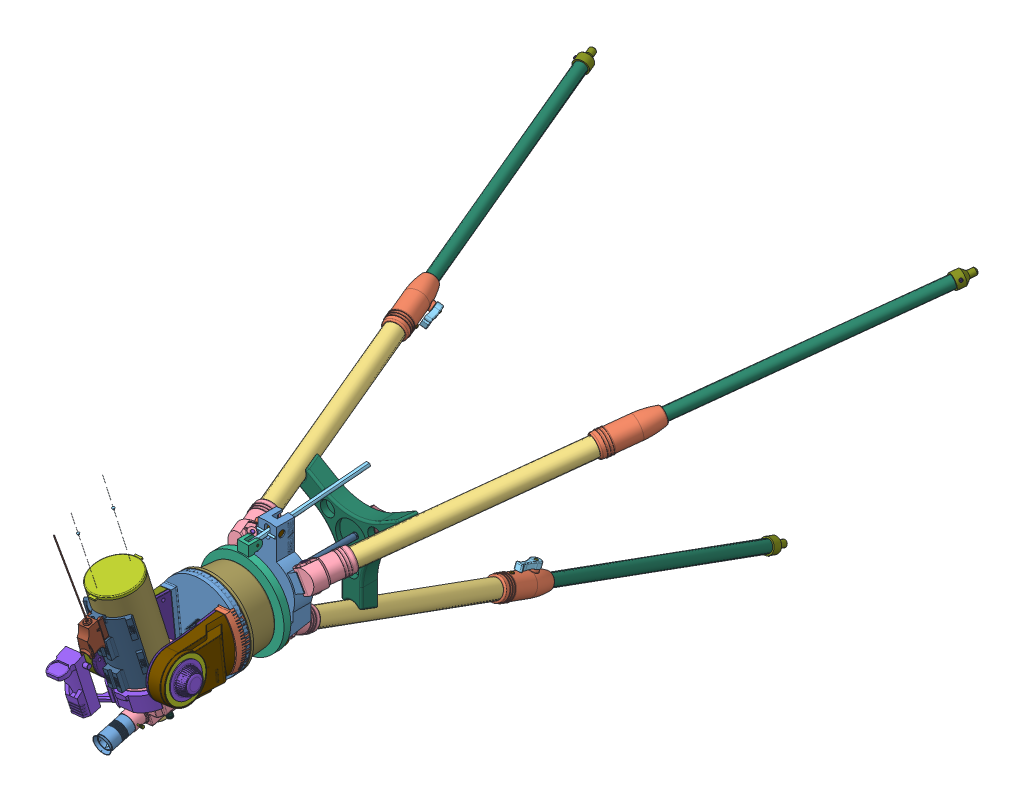
SolidWorks assembly trepied, configuration Défaut. Lengths in mm.
Overall size (885.88 767.19 1585.6).
256 component instances, 124 part files, 38 mates.
Components (placement in the parent):
- plateforme trepied-1: plateforme trepied [Défaut] at (-13.9917 -19.2932 0) size (184.28 220 78.5)
- tube superieur-1: tube superieur [Défaut] at (-47.7776 -290.931 -548.273) x (-1 0 0) z (0 -0.939693 0.34202) size (56 647 70.31)
  - liaison tube-1: liaison tube [Défaut] at (-33.7859 -53.3876 0) size (49 123 52)
  - tube superieur-1: tube superieur [Défaut] at (-33.7859 -3.3876 0) x (1 0 0) z (0 -1 0) size (38 38 530)
  - liaison tube plaque-1: liaison tube plaque [Défaut] at (-33.7859 -483.3876 0) x (-1 0 0) z (0 0 1) size (54 94 52.5)
  - manette fixation pied-1: manette fixation pied [Défaut] at (-52.9516 19.4533 -40.9) x (-1 0 0) z (0 0 1) size (22 50 29.31)
    - manette fixation pied-1: manette fixation pied [Défaut] at (-19.1657 -10.1591 0) size (22 50 15.3)
    - vis M8 fixation pied-1: vis M8 fixation pied [Défaut] at (-19.1657 -10.1591 6.2) x (1 0 0) z (0 -1 0) size (11 21.7 11)
    - Vis cr f90 M4-1: Vis cr f90 M4 [Défaut] at (-19.1657 -10.1591 1.7) size (7.4 7.4 13.11)
  - VisChcM8 50-2: VisChcM8 50 [Défaut] at (-55.5859 -557.3876 0) x (0 0 -1) z (1 0 0) size (12.3 12.3 56)
  - Vis cr M5-1: Vis cr M5 [Défaut] at (-33.7859 -20.3876 -23.15) x (0 1 0) z (0 0 1) size (7.7 7.7 9.33)
  - Vis cr M5-2: Vis cr M5 [Défaut] at (-33.7859 -516.3876 -23.15) size (7.7 7.7 9.33)
- axe M12-1: axe M12 [Défaut] at (-13.9917 -19.2932 0) x (-0.923728 -0.383049 0) z (0 0 -1) size (12.15 12.3 255.78)
- rondelle 30-1: rondelle 30 [Défaut] at (-13.9917 -19.2932 -220.4136) x (0.988696 -0.149935 0) z (0 0 1) size (30 30 2.3)
- Ecrou hexagonal ISO 4032, M 12-1: Ecrou hexagonal ISO 4032, M 12 [Défaut] at (-13.9917 -19.2932 -29.8) x (0.5 0.866025 0) z (0.866025 -0.5 0) size (20.78 10.8 18)
- ecrou plastic M12-1: ecrou plastic M12 [Défaut] at (-30.5314 -30.6977 -251.8636) x (-0.809017 -0.587785 0) z (0 0 1) size (58 55.29 30.73)
  - ecrou plastic-1: ecrou plastic [Défaut] at (-20.0843 0.4954 0) size (58 55.29 30)
  - insert M12-1: insert M12 [Défaut] at (-20.0843 0.4954 14.3) size (16 16 17.46)
- pied-1: pied [Défaut] at (-11.1207 -290.7802 -547.9154) x (1 0 0) z (0 -0.34202 -0.939693) size (30.8 33.14 626.85)
  - tube inferieur-1: tube inferieur [Défaut] at (-2.871 0.0194 0) size (25 25 600)
  - pied-1: pied [Défaut] at (-2.871 0.0194 582.85) x (1 0 0) z (0 -1 0) size (30.8 44 30.8)
  - Vis cr M4-1: Vis cr M4 [Défaut] at (-2.871 15.3194 591.85) x (0 0 -1) z (0 -1 0) size (6.7 6.7 12.44)
- pied-2: pied [Défaut] at (-250.5418 113.9639 -547.9154) x (-0.5 -0.866025 0) z (-0.296198 0.17101 -0.939693) size (30.8 33.14 626.85)
  - tube inferieur-1: tube inferieur [Défaut] at (-2.871 0.0194 0) size (25 25 600)
  - pied-1: pied [Défaut] at (-2.871 0.0194 582.85) x (1 0 0) z (0 -1 0) size (30.8 44 30.8)
  - Vis cr M4-1: Vis cr M4 [Défaut] at (-2.871 15.3194 591.85) x (0 0 -1) z (0 -1 0) size (6.7 6.7 12.44)
- pied-3: pied [Défaut] at (219.6874 118.9366 -547.9154) x (-0.5 0.866025 0) z (0.296198 0.17101 -0.939693) size (30.8 33.14 626.85)
  - tube inferieur-1: tube inferieur [Défaut] at (-2.871 0.0194 0) size (25 25 600)
  - pied-1: pied [Défaut] at (-2.871 0.0194 582.85) x (1 0 0) z (0 -1 0) size (30.8 44 30.8)
  - Vis cr M4-1: Vis cr M4 [Défaut] at (-2.871 15.3194 591.85) x (0 0 -1) z (0 -1 0) size (6.7 6.7 12.44)
- tube superieur-2: tube superieur [Défaut] at (-232.344 145.7851 -548.273) x (0.5 0.866025 0) z (-0.813798 0.469846 0.34202) size (56 647 70.31)
  - liaison tube-1: liaison tube [Défaut] at (-33.7859 -53.3876 0) size (49 123 52)
  - tube superieur-1: tube superieur [Défaut] at (-33.7859 -3.3876 0) x (1 0 0) z (0 -1 0) size (38 38 530)
  - liaison tube plaque-1: liaison tube plaque [Défaut] at (-33.7859 -483.3876 0) x (-1 0 0) z (0 0 1) size (54 94 52.5)
  - manette fixation pied-1: manette fixation pied [Défaut] at (-52.9516 19.4533 -40.9) x (-1 0 0) z (0 0 1) size (22 50 29.31)
    - manette fixation pied-1: manette fixation pied [Défaut] at (-19.1657 -10.1591 0) size (22 50 15.3)
    - vis M8 fixation pied-1: vis M8 fixation pied [Défaut] at (-19.1657 -10.1591 6.2) x (1 0 0) z (0 -1 0) size (11 21.7 11)
    - Vis cr f90 M4-1: Vis cr f90 M4 [Défaut] at (-19.1657 -10.1591 1.7) size (7.4 7.4 13.11)
  - VisChcM8 50-2: VisChcM8 50 [Défaut] at (-55.5859 -557.3876 0) x (0 0 -1) z (1 0 0) size (12.3 12.3 56)
  - Vis cr M5-1: Vis cr M5 [Défaut] at (-33.7859 -20.3876 -23.15) x (0 1 0) z (0 0 1) size (7.7 7.7 9.33)
  - Vis cr M5-2: Vis cr M5 [Défaut] at (-33.7859 -516.3876 -23.15) size (7.7 7.7 9.33)
- tube superieur-3: tube superieur [Défaut] at (238.1464 87.2662 -548.273) x (0.5 -0.866025 0) z (0.813798 0.469846 0.34202) size (56 647 70.31)
  - liaison tube-1: liaison tube [Défaut] at (-33.7859 -53.3876 0) size (49 123 52)
  - tube superieur-1: tube superieur [Défaut] at (-33.7859 -3.3876 0) x (1 0 0) z (0 -1 0) size (38 38 530)
  - liaison tube plaque-1: liaison tube plaque [Défaut] at (-33.7859 -483.3876 0) x (-1 0 0) z (0 0 1) size (54 94 52.5)
  - manette fixation pied-1: manette fixation pied [Défaut] at (-52.9516 19.4533 -40.9) x (-1 0 0) z (0 0 1) size (22 50 29.31)
    - manette fixation pied-1: manette fixation pied [Défaut] at (-19.1657 -10.1591 0) size (22 50 15.3)
    - vis M8 fixation pied-1: vis M8 fixation pied [Défaut] at (-19.1657 -10.1591 6.2) x (1 0 0) z (0 -1 0) size (11 21.7 11)
    - Vis cr f90 M4-1: Vis cr f90 M4 [Défaut] at (-19.1657 -10.1591 1.7) size (7.4 7.4 13.11)
  - VisChcM8 50-2: VisChcM8 50 [Défaut] at (-55.5859 -557.3876 0) x (0 0 -1) z (1 0 0) size (12.3 12.3 56)
  - Vis cr M5-1: Vis cr M5 [Défaut] at (-33.7859 -20.3876 -23.15) x (0 1 0) z (0 0 1) size (7.7 7.7 9.33)
  - Vis cr M5-2: Vis cr M5 [Défaut] at (-33.7859 -516.3876 -23.15) size (7.7 7.7 9.33)
- axe reglage altitude-1: axe reglage altitude [Défaut] at (-13.9917 85.0832 -12) x (0 0.996406 0.08471) z (-1 0 0) size (14 14 35)
- VisM8 15 reglage montage equatorial-1: VisM8 15 reglage montage equatorial [Défaut] at (-38.162 60.6802 -12.4568) x (0 -0.999825 -0.018716) z (0 0.018716 -0.999825) size (48.14 28.09 16.29)
  - languette-1: languette [Défaut] at (-24.4073 4.8297 0) size (45 10 2.8)
  - VisM8 15 reglage montage equatorial-1: VisM8 15 reglage montage equatorial [Défaut] at (-24.4073 -3.1703 0) x (0 0 1) z (0 -1 0) size (12 12 28.09)
  - CHCM3-10-1: CHCM3-10 [Défaut] at (-24.4073 4.8297 6.5) x (-1 0 0) z (0 0 -1) size (5 5 12.5)
  - rondelle 16-1: rondelle 16 [Défaut] at (-24.4073 -3.1703 0) x (0.999837 0 -0.018032) z (0 -1 0) size (16 16 1)
- regle-1: regle [Défaut] at (-13.9917 102.8714 -221.2334) x (1 0 0) z (0 -0.08471 0.996406) size (40 8.8 260)
- plateau inclinable-1: plateau inclinable [Défaut] at (-13.9917 5.5703 55.6) x (0 1 0) z (0 0 -1) size (206.4 185 50.37)
  - plateau inclinable-1: plateau inclinable [Défaut] at (-28.5 -0.1435 0) size (206.4 185 37.6)
  - Vis  M6-24-1: Vis  M6-24 [Défaut] at (75.7 -11.9435 22.75) x (-1 0 0) z (0 1 0) size (6 6 24)
  - rondelle 16-7: rondelle 16 [Défaut] at (-81.5 62.9965 28.6) x (-0.476926 0 0.878943) z (0 1 0) size (16 16 1)
  - rondelle 16-8: rondelle 16 [Défaut] at (-81.5 48 28.6) x (-0.476926 0 0.878943) z (0 1 0) size (16 16 1)
  - rondelle 16-9: rondelle 16 [Défaut] at (-81.5 56 28.6) x (-0.476926 0 0.878943) z (0 1 0) size (16 16 1)
  - rondelle 16-10: rondelle 16 [Défaut] at (-81.5 -56.2835 28.6) x (0.476926 0 -0.878943) z (0 -1 0) size (16 16 1)
  - rondelle 16-11: rondelle 16 [Défaut] at (-81.5 -48 28.6) x (0.476926 0 -0.878943) z (0 -1 0) size (16 16 1)
  - rondelle 16-12: rondelle 16 [Défaut] at (-81.5 -63.2835 28.6) x (0.476926 0 -0.878943) z (0 -1 0) size (16 16 1)
  - EcrouH8 nylstop-1: EcrouH8 nylstop [Défaut] at (-81.5 -48 28.6) x (0 0 -1) z (0 -1 0) size (13 15.01 7.1)
  - EcrouH8 nylstop-2: EcrouH8 nylstop [Défaut] at (-81.5 48 28.6) x (0 0 1) z (0 1 0) size (13 15.01 7.1)
  - VisHm8_25-1: VisHm8_25 [Défaut] at (-81.5 -64.2835 28.6) x (0.866025 0 0.5) z (0 1 0) size (13 15.01 29.5)
  - VisHm8_25-2: VisHm8_25 [Défaut] at (-81.5 63.9965 28.6) x (-0.866025 0 -0.5) z (0 -1 0) size (13 15.01 29.5)
  - vis plastique M6-1: vis plastique M6 [Défaut] at (-89.0406 -5.4634 33.1) x (-0.885007 -0.465577 0) z (0 0 -1) size (33.9 32.72 44.02)
    - bouton plastic-1: bouton plastic [Défaut] at (-10.2565 0.6155 0) size (33.9 32.72 15)
    - Vis  M6 30-1: Vis  M6 30 [Défaut] at (-10.2565 0.6155 15) x (-0.5 0.866025 0) z (0 0 1) size (10 11.55 34.02)
    - rondelle 12-1: rondelle 12 [Défaut] at (-10.2565 0.6155 32.1) size (11.9 11.9 1)
    - Truac-1: Truac [Défaut] at (-10.2565 0.6155 33.1) x (0 0 1) z (-0.309017 0.951057 0) size (0.6 8.54 9)
    - Ressort de compression, 9x0,4-1: Ressort de compression, 9x0,4 [Défaut] at (-10.2565 0.6155 32.1) x (0 0 -1) z (0.885007 0.465577 0) size (11.52 9.7 9.88)
  - vis plastique M6-2: vis plastique M6 [Défaut] at (14.4594 -5.4634 33.1) x (-0.885007 -0.465577 0) z (0 0 -1) size (33.9 32.72 44.02)
    - bouton plastic-1: bouton plastic [Défaut] at (-10.2565 0.6155 0) size (33.9 32.72 15)
    - Vis  M6 30-1: Vis  M6 30 [Défaut] at (-10.2565 0.6155 15) x (-0.5 0.866025 0) z (0 0 1) size (10 11.55 34.02)
    - rondelle 12-1: rondelle 12 [Défaut] at (-10.2565 0.6155 32.1) size (11.9 11.9 1)
    - Truac-1: Truac [Défaut] at (-10.2565 0.6155 33.1) x (0 0 1) z (-0.309017 0.951057 0) size (0.6 8.54 9)
    - Ressort de compression, 9x0,4-1: Ressort de compression, 9x0,4 [Défaut] at (-10.2565 0.6155 32.1) x (0 0 -1) z (0.885007 0.465577 0) size (11.52 9.7 9.88)
- cale-1: cale [Défaut] at (-13.9917 -19.2932 -219.2636) size (261.88 228.05 35)
- meade-1: meade [Défaut] at (-14.1353 -22.9297 136) x (0 -1 0) z (-1 0 0) size (501.96 412.65 282.97)
  - fourche-1: fourche [Défaut] at (-637.6539 13.0791 484.13) x (0.045417 -0.017413 0.998816) z (-0.998966 0.001172 0.045444) size (198.85 238.33 188.61)
    - branche equilibrage-1: branche equilibrage [Défaut] at (-444.0293 45.9192 -837.0232) x (0.999848 0.017413 0.00001) z (0.00001 -0.001172 0.999999) size (42.16 177.75 110.07)
    - Plaque carter équilibrage-1: Plaque carter équilibrage [Défaut] at (-443.0317 45.9366 -837.0903) x (0.999848 0.017413 0.00001) z (0.00001 -0.001172 0.999999) size (27.56 165.18 109.18)
    - Plaque carter équilibrage-2: Plaque carter équilibrage [Défaut] at (-468.0617 45.0668 -480.7137) x (-0.999848 -0.017413 -0.00001) z (-0.00001 0.001172 -0.999999) size (27.56 165.18 109.18)
    - branche motorisée-1: branche motorisée [Défaut] at (-441.716 45.9434 -837.1795) x (0.999848 0.017413 0.00001) z (0.00001 -0.001172 0.999999) size (49.59 177.72 110.04)
    - PIED DE fourche-1: PIED DE fourche [Défaut] at (-454.4692 -14.4541 -658.8869) x (0.999848 0.017413 0.00001) z (0.00001 -0.001172 0.999999) size (191.94 35.1 188.57)
      - Pied de fourche-1: Pied de fourche [Défaut] at (12.1809 59.9857 -178.2534) size (191.94 35.1 188.57)
      - Pied de fourche1-1: Pied de fourche1 [Défaut] at (-12.1809 59.9857 178.0188) x (-1 0 0) z (0 0 -1) size (54.8 35.1 115.86)
    - rondelle vis m8_50-1: rondelle vis m8_50 [Défaut] at (-454.2843 -25.0712 -659.0167) x (0.997592 0.017452 -0.067129) z (0.017413 -0.999848 -0.001172) size (26.8 26.16 7)
    - VisHM8_50-1: VisHM8_50 [Défaut] at (-454.3818 -19.4721 -659.0102) x (0.997592 0.017452 -0.067129) z (0.017413 -0.999848 -0.001172) size (12.6 14.55 55.47)
    - limiteur de couple embase-1: limiteur de couple embase [Défaut] at (-453.5008 -70.0544 -659.0694) x (0.06714 0 0.997744) z (-0.997592 -0.017452 0.067129) size (25.3 5 25.3)
    - Roue à denture hélicoïdale m=0,5 Z=60-1: Roue à denture hélicoïdale m=0,5 Z=60 [Défaut] at (-453.6431 -61.8856 -659.0599) x (0.201032 0.002353 0.979582) z (-0.017413 0.999848 0.001172) size (31.07 31.07 6.34)
    - Levier de débrayage-1: Levier de débrayage [Défaut] at (-491.4971 43.1006 -833.8173) x (0.963244 0.01709 -0.268082) z (0.268062 0.003539 0.963395) size (36.12 10 38.96)
    - plateau-1: plateau [Défaut] at (-454.3861 -19.2221 -659.0099) x (-0.997592 -0.017452 0.067129) z (0.017413 -0.999848 -0.001172) size (170 170 47)
    - EcrouHM 20-2: EcrouHM 20 [Défaut] at (-453.9456 -44.5183 -659.0395) x (0.06714 0 0.997744) z (-0.017413 0.999848 0.001172) size (30 34.64 12)
    - motoreducteur fourche-1: motoreducteur fourche [Défaut] at (-542.1299 45.8782 -641.824) x (0.06714 0 0.997744) z (0.997592 0.017452 -0.067129) size (70.5 139.71 33.06)
      - rep. 01 pignon arbre moteur + disque-1: rep. 01 pignon arbre moteur + disque [Défaut] at (0 -0.36 0) size (19 10.8 19)
      - rep. 02-03 roue Z56-1: rep. 02-03 roue Z56 [Défaut] at (0.8779 -0.6486 0.8082) x (0.995701 0 0.092628) z (-0.092628 0 0.995701) size (28.76 10.95 28.76)
      - rep. 08-09 roue inter-1: rep. 08-09 roue inter [Défaut] at (-0.15 -0.2381 0) x (1 0 0) z (0 0 1) size (12.96 5.74 12.96)
      - rep. 06-07 roue inter-1: rep. 06-07 roue inter [Défaut] at (-0.15 -0.0981 0) x (1 0 0) z (0 0 1) size (13 5.74 13)
      - rep. 04-05 roue inter-1: rep. 04-05 roue inter [Défaut] at (-21.6079 -0.6386 5.1059) x (0.907401 0 -0.420265) z (0.420265 0 0.907401) size (13 5.74 13)
      - bati-1: bati [Défaut] at (103.3128 129.885 -87.3106) size (70.5 138.91 24)
        - Axe Rep19bis-1: Axe Rep19bis [Défaut] at (-92.1856 -130.245 98.2871) x (-0.137137 0 0.990552) z (-0.990552 0 -0.137137) size (3 14 3)
        - moteur-1: moteur [Défaut] at (-103.3128 -129.885 87.3106) size (18 46.5 24)
        - axe-1: axe [Défaut] at (-111.605 -120.0821 97.7106) x (0.934599 0 -0.355704) z (0 -1 0) size (3 3 39)
        - bati2-1: bati2 [Défaut] at (-77.4849 -277.8736 138.6581) x (1 0 0) z (0 0 -1) size (17.4 55.11 17.4)
          - rondelle alu-1: rondelle alu [Défaut] at (-55.9783 -35.2009 30.6529) size (17.4 2.5 17.4)
          - Rondelle M6_1-1: Rondelle M6_1 [Défaut] at (-55.9783 -35.2009 30.6529) size (16.67 2.55 16.67)
          - rondelle alu_1-1: rondelle alu_1 [Défaut] at (-55.9783 -35.2009 30.6529) size (17.4 2.5 17.4)
          - Entretoise_1-1: Entretoise_1 [Défaut] at (-55.9783 -35.2009 30.6529) size (16.5 6 16.5)
          - Entretoise-1: Entretoise [Défaut] at (-55.9783 -35.2009 30.6529) size (16.5 6 16.5)
          - Rondelle M6-1: Rondelle M6 [Défaut] at (-55.9783 -35.2009 30.6529) size (16.67 2.55 16.67)
          - rep. 16 Ecrou M6-1: rep. 16 Ecrou M6 [Défaut] at (18.5294 -120.4752 48.0628) x (-0.896454 0 -0.443136) z (-0.443136 0 0.896454) size (12.68 6 11.39)
        - corps1-1: corps1 [Défaut] at (-126.5989 -147.7633 97.7106) size (62.7 74.5 12)
        - corps2-1: corps2 [Défaut] at (-126.5989 -147.7633 85.7106) size (62.7 50 12) (hidden)
        - châpe en alu-1: châpe en alu [Défaut] at (-133.4632 -157.3984 87.2051) size (33.3 38 19.61)
      - vis-1: vis [Défaut] at (7.3554 -71.4832 9.6533) x (1 0 0) z (0 1 0) size (33.09 33.06 82.71)
        - Vis san fin m=0,5 - 1 filet(s)-2: Vis san fin m=0,5 - 1 filet(s) [Défaut] at (-0.6479 -0.6412 0.3804) x (0.7262 -0.687484 0) z (0 0 1) size (8.16 8.16 68.9)
        - rep12-4: rep12 [Défaut] at (-11.6724 36.0347 43.7266) x (0.537117 -0.843508 0) z (-0.843508 -0.537117 0) size (23.91 29.81 24)
      - engrenage-1: engrenage [Défaut] at (-45.9983 -125.8694 31.0757) x (-0.919401 0 0.393321) z (0.393321 0 0.919401) size (12.99 17.44 12.99)
        - rep.11SLDPRT-1: rep.11SLDPRT [Défaut] at (-64.557 -106.8565 -14.5787) size (9.52 16 9.52)
        - rep. yacine-1: rep. yacine [Défaut] at (-64.557 -106.8565 -14.5787) size (12.99 1.44 12.99)
      - Vis à tête cylindrique à six pans creux Chc M2,5 - 8-1: Vis à tête cylindrique à six pans creux Chc M2,5 - 8 [Défaut] at (6.7074 -20.6971 10.2945) x (0.636786 0 0.771041) z (0 -1 0) size (4.2 4.2 10.57)
      - joint 9 5 emb-1: joint 9 5 emb [Défaut] at (6.7074 -89.1506 10.2945) size (13.5 2 13.5)
      - joint 9 5 emb-2: joint 9 5 emb [Défaut] at (6.7074 -53.1506 10.2945) size (13.5 2 13.5)
    - Vis sans tête à six pans creux à bout cuvette M3 - 3-1: Vis sans tête à six pans creux à bout cuvette M3 - 3 [Réaliste] at (-445.1418 -17.1499 -659.6319) x (-0.019293 -0.859815 -0.51024) z (0.066624 -0.510307 0.857408) size (3.03 3.08 3.04)
    - Vis à tête cylindrique bombée cruciforme type H M3 - 10-1: Vis à tête cylindrique bombée cruciforme type H M3 - 10 [Filetage Réaliste] at (-521.841 56.7793 -695.504) x (-0.997592 -0.017452 0.067129) z (-0.0364 0.955572 -0.292501) size (12.58 5.6 5.6)
    - Vis à tête cylindrique bombée cruciforme type H M3 - 10-2: Vis à tête cylindrique bombée cruciforme type H M3 - 10 [Filetage Réaliste] at (-508.9533 16.8988 -611.179) x (-0.997592 -0.017452 0.067129) z (-0.040277 -0.642181 -0.765494) size (12.58 5.6 5.6)
    - Vis à tête cylindrique bombée cruciforme type H M3 - 10-3: Vis à tête cylindrique bombée cruciforme type H M3 - 10 [Filetage Réaliste] at (-514.8616 16.8988 -698.9804) x (-0.997592 -0.017452 0.067129) z (-0.068087 0.06176 -0.995766) size (12.58 5.6 5.6)
    - Vis à tête cylindrique bombée cruciforme type H M3 - 10-4: Vis à tête cylindrique bombée cruciforme type H M3 - 10 [Filetage Réaliste] at (-521.2936 154.7556 -654.4481) x (-0.997592 -0.017452 0.067129) z (-0.06714 0 -0.997744) size (12.58 5.6 5.6)
    - Vis à tête cylindrique bombée cruciforme type H M3 - 10-5: Vis à tête cylindrique bombée cruciforme type H M3 - 10 [Filetage Réaliste] at (-516.3356 56.7793 -613.689) x (-0.997592 -0.017452 0.067129) z (-0.06714 0 -0.997744) size (12.58 5.6 5.6)
    - Vis à tête cylindrique bombée cruciforme type H M3 - 10-7: Vis à tête cylindrique bombée cruciforme type H M3 - 10 [Filetage Réaliste] at (-393.6444 157.0051 -663.0973) x (0.997592 0.017452 -0.067129) z (0.06714 0 0.997744) size (12.58 5.6 5.6)
    - Vis à tête cylindrique bombée cruciforme type H M3 - 10-8: Vis à tête cylindrique bombée cruciforme type H M3 - 10 [Filetage Réaliste] at (-401.1787 18.9039 -706.6898) x (0.997592 0.017452 -0.067129) z (0.06714 0 0.997744) size (12.58 5.6 5.6)
    - Vis à tête cylindrique bombée cruciforme type H M3 - 10-10: Vis à tête cylindrique bombée cruciforme type H M3 - 10 [Filetage Réaliste] at (-395.1895 59.0113 -704.086) x (0.997592 0.017452 -0.067129) z (0.06714 0 0.997744) size (12.58 5.6 5.6)
    - Vis à tête cylindrique fendue CS M4 - 10-1: Vis à tête cylindrique fendue CS M4 - 10 [Défaut] at (-539.7157 125.5672 -628.3483) x (0.067415 -0.016315 0.997592) z (-0.997592 -0.017452 0.067129) size (7 7 10.62)
    - Vis à tête cylindrique fendue CS M4 - 10-2: Vis à tête cylindrique fendue CS M4 - 10 [Défaut] at (-538.2089 116.0774 -615.8713) x (0.067415 -0.016315 0.997592) z (-0.997592 -0.017452 0.067129) size (7 7 10.62)
    - Vis à tête cylindrique fendue CS M4 - 10-3: Vis à tête cylindrique fendue CS M4 - 10 [Défaut] at (-539.3849 106.5701 -628.3705) x (0.067415 -0.016315 0.997592) z (-0.997592 -0.017452 0.067129) size (7 7 10.62)
    - Vis à tête cylindrique bombée cruciforme type H M3 - 12-2: Vis à tête cylindrique bombée cruciforme type H M3 - 12 [Filetage Réaliste] at (-395.2704 18.9039 -618.8883) x (0.997592 0.017452 -0.067129) z (0.067129 0.000586 0.997744) size (14.59 5.6 5.6)
    - Vis à tête cylindrique bombée cruciforme type H M3 - 12-3: Vis à tête cylindrique bombée cruciforme type H M3 - 12 [Filetage Réaliste] at (-389.684 59.0113 -622.271) x (0.997592 0.017452 -0.067129) z (0.068185 -0.42423 0.902984) size (14.59 5.6 5.6)
    - Vis à tête cylindrique bombée cruciforme type H M3 - 25-1: Vis à tête cylindrique bombée cruciforme type H M3 - 25 [Filetage Réaliste] at (-516.5693 58.6063 -628.1014) x (-0.997592 -0.017452 0.067129) z (-0.067129 0.486457 -0.871122) size (32.61 5.6 5.6)
    - Vis à tête cylindrique bombée cruciforme type H M3 - 25-2: Vis à tête cylindrique bombée cruciforme type H M3 - 25 [Filetage Réaliste] at (-520.3322 72.7741 -680.3366) x (-0.997592 -0.017452 0.067129) z (-0.067129 0.486457 -0.871122) size (32.61 5.6 5.6)
    - Vis à tête cylindrique bombée cruciforme type H M3 - 25-3: Vis à tête cylindrique bombée cruciforme type H M3 - 25 [Filetage Réaliste] at (-519.8272 43.7786 -680.3706) x (-0.997592 -0.017452 0.067129) z (0.067053 0.00493 0.997737) size (32.61 5.6 5.6)
    - Vis à tête cylindrique bombée cruciforme type H M3 - 20-1: Vis à tête cylindrique bombée cruciforme type H M3 - 20 [Filetage Réaliste] at (-531.1265 -25.9655 -653.8459) x (-0.017413 0.999848 0.001172) z (0.998816 0.017342 0.045444) size (22.61 5.6 5.6)
    - Vis à tête cylindrique bombée cruciforme type H M3 - 20-2: Vis à tête cylindrique bombée cruciforme type H M3 - 20 [Filetage Réaliste] at (-512.8439 -25.695 -612.9812) x (-0.017413 0.999848 0.001172) z (0.998816 0.017342 0.045444) size (22.61 5.6 5.6)
    - Vis à tête cylindrique bombée cruciforme type H M3 - 20-3: Vis à tête cylindrique bombée cruciforme type H M3 - 20 [Filetage Réaliste] at (-517.7505 -25.6821 -696.841) x (-0.017413 0.999848 0.001172) z (0.998816 0.017342 0.045444) size (22.61 5.6 5.6)
    - Vis à tête cylindrique bombée cruciforme type H M3 - 20-4: Vis à tête cylindrique bombée cruciforme type H M3 - 20 [Filetage Réaliste] at (-395.7403 -23.5476 -705.0512) x (-0.017413 0.999848 0.001172) z (0.998816 0.017342 0.045444) size (22.61 5.6 5.6)
    - Vis à tête cylindrique bombée cruciforme type H M3 - 20-5: Vis à tête cylindrique bombée cruciforme type H M3 - 20 [Filetage Réaliste] at (-377.4577 -23.2771 -664.1865) x (-0.017413 0.999848 0.001172) z (0.998816 0.017342 0.045444) size (22.61 5.6 5.6)
    - Vis à tête cylindrique bombée cruciforme type H M3 - 20-6: Vis à tête cylindrique bombée cruciforme type H M3 - 20 [Filetage Réaliste] at (-390.8337 -23.5604 -621.1914) x (-0.017413 0.999848 0.001172) z (0.998816 0.017342 0.045444) size (22.61 5.6 5.6)
  - tube-1: tube [Défaut] at (-15.3759 72.4194 1.7393) x (0.112402 0 0.993663) z (-0.967198 0.229253 0.109409) size (229.47 195.18 484.9)
    - Capuchon port photo-2: Capuchon port photo [Défaut] at (20.0265 52.1414 -183.8549) x (0.753442 -0.654583 0.06202) z (-0.29492 -0.252137 0.921656) size (39.95 39.82 23.78)
    - support objectif-2: support objectif [Défaut] at (0 67.5 -76) size (179.88 130.77 134.7)
    - Palier d'embrayage-2: Palier d'embrayage [Défaut] at (24.7034 252.6163 -72.3954) x (0.997744 -0.06714 0) z (-0.06714 -0.997744 0) size (14.91 34.8 28.76)
    - palier-2: palier [Défaut] at (-93.6662 67.5 0) x (1 0 0) z (0 -0.589029 0.808112) size (10.05 25.5 25.5)
    - Roue à denture hélicoïdale m=0,5 Z=60-3: Roue à denture hélicoïdale m=0,5 Z=60 [Défaut] at (-77.15 67.5 0) x (0 0.783284 -0.621664) z (1 0 0) size (31.07 31.07 6.34)
    - Plaque repérage angulaire-3: Plaque repérage angulaire [Défaut] at (-159.1429 162.8547 -174.0321) x (0.997744 -0.051519 0.043053) z (-0.06714 -0.765605 0.639798) size (6.77 89 88.85)
    - molette blocage vertical-2: molette blocage vertical [Défaut] at (25.2373 156.4775 -169.1848) x (0.997744 -0.051429 0.043161) z (-0.06714 -0.764265 0.641398) size (31.87 70 69.98)
    - molette blocage 2 vertical-2: molette blocage 2 vertical [Défaut] at (-32.8172 155.1442 169.8822) x (-0.997741 -0.051084 -0.043619) z (0.067172 -0.759198 -0.647384) size (27.85 70 69.98)
    - Plaque repérage angulaire-4: Plaque repérage angulaire [Défaut] at (151.5627 161.1167 174.9858) x (-0.997741 -0.051084 -0.043619) z (0.067172 -0.759198 -0.647384) size (6.77 89 88.85)
    - Embout fileté-2: Embout fileté [Défaut] at (31.1097 71.2083 -217.7977) x (0.995668 0.069272 0.06202) z (-0.030498 -0.386808 0.921656) size (96.08 90.33 41.21)
    - miroir-2: miroir [Défaut] at (1.5401 49.2079 -414.2886) x (0 -0.998075 0.06202) z (-0.383759 0.057271 0.921656) size (89.51 86.43 44.67)
    - tube-2: tube [Défaut] at (0 67.5 -53.7618) x (0 0 -1) z (1 0 0) size (225 100 100)
    - menisque-2: menisque [Défaut] at (-10.827 126.3859 145.8849) x (-0.376431 0.924349 0.062271) z (0.377105 0.091483 0.921641) size (110.67 106.16 46.27)
      - menisque-1: menisque [Défaut] at (-56.116 -127.6725 -342.9742) size (27.57 28.77 19.69)
      - Piece1-1: Piece1 [Défaut] at (-57.8098 16.1933 3.3103) x (0.972599 -0.230535 0.030091) z (-0.028457 0.010411 0.999541) size (92 86.87 40.19)
    - molette-2: molette [Défaut] at (16.1783 77.4199 -201.1536) x (0.997152 -0.042906 0.06202) z (-0.073715 -0.380942 0.921656) size (12.27 29.01 54.01)
    - Vis porte oculaire-2: Vis porte oculaire [Défaut] at (70.5773 71.9334 3.0696) x (0.833291 0.517003 -0.195792) z (-0.515568 0.854579 0.062325) size (15.46 8.19 13.39)
    - bouton miroir-3: bouton miroir [Défaut] at (118.3372 40.7094 -82.3) x (0.999979 -0.006557 0) z (0 0 1) size (83.58 43.34 43.14)
      - bouton miroir-1: bouton miroir [Défaut] at (-90.8002 18.3233 -120.2299) x (0.996615 -0.012919 0.081184) z (-0.081184 -0.309873 0.947306) size (41.27 12.61 13.28)
      - bouton miroir-2: bouton miroir [Défaut] at (-145.9581 -6.2943 -120.2299) x (-0.996615 0.012919 0.081184) z (0.081184 0.309873 0.947306) size (41.27 12.61 13.28)
      - petit miroir-1: petit miroir [Défaut] at (-118.5103 26.0141 2.75) x (0.999979 0.006557 0) z (0.004637 -0.707092 0.707107) size (30 26.01 35)
    - oculaire-2: oculaire [Défaut] at (0 149.5136 -0.7045) x (0 0 1) z (-1 0 0) size (38 81.5 38)
      - oculaire-1: oculaire [Défaut] at (-78.8455 -41.743 0) size (38 81.5 38)
      - lentille-1: lentille [Défaut] at (-81.1151 5.0064 0) x (0 -1 0) z (0 0 1) size (10.53 25 25)
        - lentille 1-1: lentille 1 [Défaut] at (-6.7507 2.2696 0) size (8.01 25 25)
        - lentille 2-1: lentille 2 [Défaut] at (-12.7507 2.2696 0) size (4.52 25 25)
      - lentille-2: lentille [Défaut] at (-76.963 10.0077 1.2678) x (0 1 0) z (-0.558618 0 0.829425) size (10.53 25 25)
        - lentille 1-1: lentille 1 [Défaut] at (-6.7507 2.2696 0) size (8.01 25 25)
        - lentille 2-1: lentille 2 [Défaut] at (-12.7507 2.2696 0) size (4.52 25 25)
    - faisceau2-2: faisceau2 [Défaut] at (0 78.827 -14.9477) x (0 0 -1) z (1 0 0) size (437.42 120.49 0.34)
    - fleche-13: fleche [Défaut] at (0 108.7031 110.8339) x (0 0 1) z (-0.886861 -0.462037 0) size (8 5.6 5.6)
    - fleche-14: fleche [Défaut] at (0 88.228 83.446) x (0 0.178036 -0.984024) z (1 -0.000403 -0.000073) size (8 5.6 5.6)
    - fleche-15: fleche [Défaut] at (0 75.6322 94.3005) x (0 0.005533 0.999985) z (0.072331 0.997365 -0.005519) size (8 5.6 5.6)
    - fleche-16: fleche [Défaut] at (0 108.7103 294.2676) x (0 0.017452 0.999848) z (-0.523715 0.851763 -0.014868) size (8 5.6 5.6)
    - fleche-17: fleche [Défaut] at (0 127.4306 -74.061) x (0 -0.974863 -0.222804) z (-0.735553 0.150943 -0.660438) size (8 5.6 5.6)
    - fleche-18: fleche [Défaut] at (0 183.519 -69.8214) x (0 -1 0) z (-0.316126 0 0.948717) size (8 5.6 5.6)
    - faisceau1-2: faisceau1 [Défaut] at (0 -20.7845 -6.8996) x (0 0 -1) z (1 0 0) size (447.26 167.74 0.41)
    - fleche-19: fleche [Défaut] at (0 30.6251 284.852) x (0 0 1) z (-0.426184 0.904636 0) size (8 5.6 5.6)
    - fleche-20: fleche [Défaut] at (0 27.6512 105.4051) x (0 0 1) z (-0.740163 -0.672427 0) size (8 5.6 5.6)
    - fleche-21: fleche [Défaut] at (0 46.7601 79.6116) x (0 -0.171906 -0.985113) z (0.984293 0.173915 -0.030349) size (8 5.6 5.6)
    - fleche-22: fleche [Défaut] at (0 59.5724 94.0494) x (0 -0.005145 0.999987) z (-0.101559 -0.994816 -0.005119) size (8 5.6 5.6)
    - fleche-23: fleche [Défaut] at (0 127.1897 -84.7907) x (0 -0.982309 0.187268) z (-0.405585 0.171174 0.897887) size (8 5.6 5.6)
    - fleche-24: fleche [Défaut] at (0 183.4575 -88.3366) x (0 -1 0) z (-0.976187 0 0.216931) size (8 5.6 5.6)
    - cache-2: cache [Défaut] at (0 67.5 174.5) x (0 0 -1) z (1 0 0) size (10 111 100)
    - Module LNT-2: Module LNT [Défaut] at (0 67.5 -16) x (0.999806 -0.019718 0) z (0 0 1) size (140.9 99.11 110)
    - Vis à tête cylindrique fendue CS M3 - 10-1: Vis à tête cylindrique fendue CS M3 - 10 [Défaut] at (27 106.7707 -61.5) size (5.5 5.5 12.01)
    - telescope v5 SET PROTO-1: telescope v5 SET PROTO [Défaut] at (0 67.5 -9.3345) size (105.63 40.25 150.9)
    - Pièce1^tube-1: Pièce1^tube [Défaut] at origin (virtual)
    - POINTEUR laser-1: POINTEUR laser [Défaut] at (0.125 116.1734 142.1075) x (1 0 0) z (0 0 -1) size (28.99 45.08 248.53)
  - CARTER EMBASE-2: CARTER EMBASE [Défaut] at (-38.5593 -33.7526 0) x (-1 0 0) z (0 0 -1) size (208.81 81 208.82)
    - Carter embase-1: Carter embase [Défaut] at (-38.5593 34.3526 0) size (182.1 77.5 182)
    - palier-1: palier [Défaut] at (-38.7022 18.1339 0.128) x (-0.744983 0 0.667084) z (0.667084 0 0.744983) size (45.68 15.3 45.68)
      - palier alu-1: palier alu [Défaut] at (-0.1919 7.7813 0) size (40 13.5 40)
      - palier axial-1: palier axial [Défaut] at (-0.1919 -6.6187 0) size (33 6.3 33)
      - palier axial-2: palier axial [Défaut] at (-0.1919 8.6813 0) x (-0.837169 0 -0.546944) z (-0.546944 0 0.837169) size (33 6.3 33)
    - plaque branchement-1: plaque branchement [Défaut] at (-38.5593 -18.7385 -76.5024) x (1 0 0) z (0 0.068841 0.997628) size (62.31 43.19 20.2)
    - carter couvercle-1: carter couvercle [Défaut] at (-38.5593 -43.1474 0) x (0 0 1) z (-1 0 0) size (145 23 145)
    - anneau guide-1: anneau guide [Défaut] at (-38.5593 19.8526 0) x (-0.683843 0 0.729629) z (0 1 0) size (46.6 56.5 4.2)
    - support palier-1: support palier [Défaut] at (-38.5593 58.1532 0) x (0.258819 0 -0.965926) z (0.965926 0 0.258819) size (170.5 70.67 170.49)
    - reducteur embase-1: reducteur embase [Défaut] at (-74.9499 2.4826 -18.0358) x (0 0 1) z (0 -1 0) size (101.77 85.1 39.66)
      - rep. 01 pignon arbre moteur + disque-1: rep. 01 pignon arbre moteur + disque [Défaut] at (0.9543 -1.36 18.0797) x (0.78085 0 0.624719) z (-0.624719 0 0.78085) size (19 10.8 19)
      - rep. 02-03 roue Z56-1: rep. 02-03 roue Z56 [Défaut] at (-12.7174 -0.5 -2.1104) x (0.531735 0 -0.846911) z (0.846911 0 0.531735) size (28.76 10.95 28.76)
      - rep. 08-09 roue inter-1: rep. 08-09 roue inter [Défaut] at (-2.3943 -0.3381 0.4364) x (0.975998 0 -0.217777) z (0.217777 0 0.975998) size (12.96 5.74 12.96)
      - rep. 06-07 roue inter-1: rep. 06-07 roue inter [Défaut] at (-3.1771 0.3019 0.7148) x (0.955582 0 -0.294727) z (0.294727 0 0.955582) size (13 5.74 13)
      - roue rep 12 (petite folle)-1: roue rep 12 (petite folle) [Défaut] at (0.2679 -0.4 -0.3808) x (0.999222 0 0.039446) z (-0.039446 0 0.999222) size (13 3.24 13)
      - rep. 04-05 roue inter-1: rep. 04-05 roue inter [Défaut] at (2.2907 -0.16 -1.8606) x (0.977065 0 0.21294) z (-0.21294 0 0.977065) size (13 5.74 13)
      - bati emb-1: bati emb [Défaut] at (103.3128 129.885 -87.3106) size (101.77 84.35 25.96)
        - coque droite emb-1: coque droite emb [Défaut] at (-103.3128 -129.885 87.3106) size (93.29 54 12.58)
        - Axe Rep19bis emb-1: Axe Rep19bis emb [Défaut] at (-103.9752 -130.143 87.3656) x (0.998781 0 -0.049366) z (0.049366 0 0.998781) size (3 15.3 3)
        - Axe Rep20.bis emb-1: Axe Rep20.bis emb [Défaut] at (-97.8983 -130.0094 79.9317) x (0.927514 0 0.373788) z (-0.373788 0 0.927514) size (3 22 3)
        - coque gauche emb-1: coque gauche emb [Défaut] at (-103.3128 -129.885 87.3106) size (94.76 55 11.51)
        - axe emb-1: axe emb [Défaut] at (-111.605 -119.0221 97.7106) x (0.824702 0 -0.565567) z (0 -1 0) size (3 3 15)
        - Axe Rep19bis emb-2: Axe Rep19bis emb [Défaut] at (-101.4828 -129.945 90.8669) x (0.715658 0 -0.698451) z (0.698451 0 0.715658) size (3 15.3 3)
        - moteur-2: moteur [Défaut] at (-103.3128 -129.885 87.3106) size (18 46.5 24)
        - châpe en alu emb-2: châpe en alu emb [Défaut] at (-103.4628 -123.4884 87.3106) size (32 38 21)
        - Entretoise emb-3: Entretoise emb [Défaut] at (-100.6729 -123.5884 80.7498) x (0.982912 0 0.184074) z (-0.184074 0 0.982912) size (17.65 5.7 17.65)
        - rondelle alu emb-3: rondelle alu emb [Défaut] at (-90.9589 -123.8884 68.1548) x (0.821605 0 0.570058) z (-0.570058 0 0.821605) size (17.4 2.65 17.4)
        - rep. 16 Ecrou M6 emb-2: rep. 16 Ecrou M6 emb [Défaut] at (-102.7157 -122.485 84.9564) x (0.99792 0 0.06446) z (-0.06446 0 0.99792) size (12.68 6 11.39)
        - Rondelle M6 emb-2: Rondelle M6 emb [Défaut] at (-94.2052 -123.7384 71.161) x (0.88187 0 0.471493) z (-0.471493 0 0.88187) size (16 1.8 16)
        - joint 9 5 emb-3: joint 9 5 emb [Défaut] at (-66.605 -149.1255 97.7106) size (13.5 2 13.5)
        - joint 9 5 emb-4: joint 9 5 emb [Défaut] at (-66.605 -183.1255 97.7106) x (0.837169 0 0.546944) z (0.546944 0 -0.837169) size (13.5 2 13.5)
        - rondelle alu emb-4: rondelle alu emb [Défaut] at (-91.5165 -167.7384 68.6232) x (0.832295 0 0.554332) z (-0.554332 0 0.832295) size (17.4 2.65 17.4)
        - Entretoise emb-4: Entretoise emb [Défaut] at (-30.2975 -208.6627 109.115) x (-0.835834 0 -0.548983) z (-0.548983 0 0.835834) size (17.65 5.7 17.65)
        - Rondelle M6 emb-3: Rondelle M6 emb [Défaut] at (-29.9622 -208.5127 109.2274) x (-0.837169 0 -0.546944) z (-0.546944 0 0.837169) size (16 1.8 16)
        - Vis à tête cylindrique bombée cruciforme type H M3 - 12-1: Vis à tête cylindrique bombée cruciforme type H M3 - 12 [Filetage Réaliste] at (-110.205 -142.8221 109.7106) x (0 0 -1) z (1 0 0) size (14.59 5.6 5.6)
        - Vis à tête cylindrique bombée cruciforme type H M3 - 12-2: Vis à tête cylindrique bombée cruciforme type H M3 - 12 [Filetage Réaliste] at (-93.3519 -120.1721 111.5106) x (0 0 -1) z (-0.592827 0.80533 0) size (14.59 5.6 5.6)
      - vis emb-1: vis emb [Défaut] at (37.3558 -36.1406 9.7588) x (1 0 0) z (0 1 0) size (25.74 25.82 76.16)
        - Vis san fin m=0,5 - 1 filet(s) emb-1: Vis san fin m=0,5 - 1 filet(s) emb [Défaut] at (-0.6479 -0.6412 0) size (8.16 8.16 68.9)
        - rep12 emb-3: rep12 emb [Défaut] at (-38.2155 6.7975 36.7974) x (0.996839 0.079451 0) z (0.079451 -0.996839 0) size (23.91 23.8 24)
      - engrenage-1: engrenage [Défaut] at (64.1683 106.4565 3.5924) x (0.967334 0 -0.253504) z (0.253504 0 0.967334) size (12.99 17.44 12.99)
        - rep.11SLDPRT-1: rep.11SLDPRT [Défaut] at (-64.557 -106.8565 -14.5787) size (9.52 16 9.52)
        - rep. yacine-1: rep. yacine [Défaut] at (-64.557 -106.8565 -14.5787) size (12.99 1.44 12.99)
      - Vis à tête cylindrique à six pans creux Chc M2,5 - 8-1: Vis à tête cylindrique à six pans creux Chc M2,5 - 8 [Défaut] at (36.7078 7.7163 10.4) x (1 0 0) z (0 -1 0) size (4.2 4.2 10.57)
    - Vis à tête fraisée FS M5 - 16-1: Vis à tête fraisée FS M5 - 16 [Défaut] at (-102.5593 -40.456 0) x (-1 0 0) z (0 1 0) size (10.32 10.4 16)
    - Vis à tête fraisée FS M5 - 16-2: Vis à tête fraisée FS M5 - 16 [Défaut] at (-6.5593 -40.456 55.4256) x (0.5 0 0.866025) z (0 1 0) size (10.32 10.4 16)
    - Vis à tête fraisée FS M5 - 16-3: Vis à tête fraisée FS M5 - 16 [Défaut] at (-6.5593 -40.456 -55.4256) x (0.5 0 -0.866025) z (0 1 0) size (10.32 10.4 16)
    - Vis à tête cylindrique bombée cruciforme type H M3 - 12-1: Vis à tête cylindrique bombée cruciforme type H M3 - 12 [Filetage Réaliste] at (-58.5127 -18.1174 -56.178) x (0 1 0) z (0 0 1) size (14.59 5.6 5.6)
    - Vis à tête cylindrique bombée cruciforme type H M3 - 12-2: Vis à tête cylindrique bombée cruciforme type H M3 - 12 [Filetage Réaliste] at (-89.2627 -18.7174 28.322) x (0 1 0) z (0 0 1) size (14.59 5.6 5.6)
    - Vis à tête cylindrique fendue CS M4 - 10-1: Vis à tête cylindrique fendue CS M4 - 10 [Défaut] at (-38.4593 -1.6174 37.562) x (1 0 0) z (0 1 0) size (7 7 10.62)
    - Vis à tête cylindrique fendue CS M4 - 10-2: Vis à tête cylindrique fendue CS M4 - 10 [Défaut] at (-31.0593 -0.5174 24.912) x (1 0 0) z (0 1 0) size (7 7 10.62)
    - Vis à tête cylindrique fendue CS M4 - 10-3: Vis à tête cylindrique fendue CS M4 - 10 [Défaut] at (-45.8593 -0.5174 24.912) x (1 0 0) z (0 1 0) size (7 7 10.62)
Mates (geometry in assembly coordinates):
- Coïncidente1: coincident anti-aligned: plane of plateforme trepied-1 through (-13.9917 -19.2932 0) normal (1 0 0); plane of tube superieur-1/liaison tube-1
- Coïncidente2: coincident: plane of plateforme trepied-1 through (-13.9917 -99.2932 0) normal (0 -1 0); axis of tube superieur-1/liaison tube plaque-1 through (-31.9917 -99.2932 -23) axis (1 0 0)
- Coaxiale2: concentric aligned: cylinder of plateforme trepied-1 through (4.0083 -100.2932 -24.5) axis (-1 0 0) radius 4; cylinder of tube superieur-1/VisChcM8 50-2 through (7.8083 -100.2932 -24.5) axis (-1 0 0) radius 4
- Coïncidente4: coincident: plane of plateforme trepied-1 through (4.0083 -93.7932 -8) normal (0 0 1); line of tube superieur-1/liaison tube plaque-1 through (-31.9917 -97.3892 -7.7499) axis (1 0 0)
- Angle1: planar angle = 0.349066 rad aligned: axis of plateforme trepied-1 through (-13.9917 -19.2932 -5) axis (0 0 -1); axis of tube superieur-1/liaison tube plaque-1 through (-13.9917 -108.5017 -47.0526) axis (0 -0.34202 -0.939693)
- Coaxiale3: concentric aligned: cylinder of plateforme trepied-1 through (-13.9917 -19.2932 -19) axis (0 0 -1) radius 5.1; cylinder of axe M12-1 through (-13.9917 -19.2932 0) axis (0 0 -1) radius 6
- Coïncidente6: coincident aligned: plane of plateforme trepied-1 through (-13.9917 -19.2932 0) normal (0 0 1); plane of axe M12-1 through (-13.9917 -19.2932 0) normal (0 0 1)
- Coaxiale4: concentric anti-aligned: cylinder of axe M12-1 through (-13.9917 -19.2932 0) axis (0 0 -1) radius 6; cylinder of Ecrou hexagonal ISO 4032, M 12-1 through (-13.9917 -19.2932 -27.4) axis (0 0 1) radius 4.4845
- Coïncidente7: coincident anti-aligned: plane of plateforme trepied-1 through (-13.9917 -19.2932 -19) normal (0 0 -1); plane of Ecrou hexagonal ISO 4032, M 12-1 through (-11.7495 -15.4096 -19) normal (0 0 1)
- Parallèle2: parallel aligned: plane of plateforme trepied-1 through (-69.9917 -79.2932 -40) normal (0 -1 0); plane of Ecrou hexagonal ISO 4032, M 12-1 through (-8.7956 -28.2932 -19) normal (0 -1 0)
- Coaxiale5: concentric aligned: cylinder of axe M12-1 through (-13.9917 -19.2932 0) axis (0 0 -1) radius 6; cylinder of rondelle 30-1 through (-13.9917 -19.2932 -219.2636) axis (0 0 -1) radius 6.75
- Coaxiale6: concentric anti-aligned: cylinder of axe M12-1 through (-13.9917 -19.2932 0) axis (0 0 -1) radius 6; cylinder of ecrou plastic M12-1/ecrou plastic-1 through (-13.9917 -19.2932 -251.8646) axis (0 0 1) radius 12.5
- Coaxiale7: concentric anti-aligned: cylinder of tube superieur-1/tube superieur-1 through (-13.9917 -108.5017 -47.0526) axis (0 -0.34202 -0.939693) radius 19; cylinder of pied-1/tube inferieur-1 through (-13.9917 -496.0105 -1111.7244) axis (0 0.34202 0.939693) radius 12.5
- Distance1: distance = 70 mm anti-aligned: plane of pied-1/tube inferieur-1 through (-13.9917 -290.7985 -547.9088) normal (0 0.34202 0.939693); plane of tube superieur-1/liaison tube-1 through (-30.4917 -314.7399 -613.6873) normal (0 -0.34202 -0.939693)
- Angle2: planar angle = 0.349066 rad aligned: axis of tube superieur-1/liaison tube plaque-1 through (-13.9917 -108.5017 -47.0526) axis (0 -0.34202 -0.939693); axis of axe M12-1 through (-13.9917 -19.2932 0) axis (0 0 -1)
- Coaxiale8: concentric anti-aligned: cylinder of axe reglage altitude-1 through (-31.4917 85.0832 -12) axis (1 0 0) radius 7; cylinder of VisM8 15 reglage montage equatorial-1/VisM8 15 reglage montage equatorial-1 through (-34.9917 85.0832 -12) axis (-1 0 0) radius 6
- Coïncidente35: coincident anti-aligned: plane of plateforme trepied-1 through (-33.9917 103.0832 -40) normal (-1 0 0); plane of VisM8 15 reglage montage equatorial-1/rondelle 16-1 through (-33.9917 85.0832 -12) normal (1 0 0)
- Coaxiale9: concentric anti-aligned: cylinder of plateforme trepied-1 through (46.0083 85.0832 -12) axis (-1 0 0) radius 7; cylinder of axe reglage altitude-1 through (-31.4917 85.0832 -12) axis (1 0 0) radius 7
- Coïncidente12: coincident anti-aligned: plane of plateforme trepied-1 through (-13.9917 -19.2932 0) normal (1 0 0); plane of axe reglage altitude-1 through (-13.9917 85.0832 -12) normal (-1 0 0)
- Coaxiale10: concentric aligned: cylinder of axe reglage altitude-1 through (-13.9917 84.4903 -5.0252) axis (0 0.08471 -0.996406) radius 5; cylinder of regle-1 through (-13.9917 80.8467 37.832) axis (0 0.08471 -0.996406) radius 5
- Coaxiale11: concentric anti-aligned: cylinder of regle-1 through (-18.9917 81.2703 32.85) axis (1 0 0) radius 2.5; cylinder of plateau inclinable-1/Vis  M6-24-1 through (-7.9353 81.2703 32.85) axis (-1 0 0) radius 2.375
- Coïncidente13: coincident aligned: plane of regle-1; plane of plateau inclinable-1
- Parallèle3: parallel aligned: plane of plateforme trepied-1 through (6.0083 103.0832 -40) normal (1 0 0); plane of plateau inclinable-1/plateau inclinable-1 through (-1.9353 81.2703 31.75) normal (1 0 0)
- Coaxiale15: concentric aligned: cylinder of plateforme trepied-1 through (35.0083 -75.9297 27) axis (1 0 0) radius 4.25; cylinder of plateau inclinable-1/plateau inclinable-1 through (43.0047 -75.9297 27) axis (1 0 0) radius 4.25
- Coïncidente21: coincident anti-aligned: plane of plateforme trepied-1 through (35.0083 -9.7694 -5) normal (-1 0 0); plane of plateau inclinable-1/rondelle 16-8 through (35.0083 -75.9297 27) normal (1 0 0)
- Coïncidente22: coincident anti-aligned: plane of plateforme trepied-1 through (42.0083 -79.2932 -40) normal (1 0 0); plane of plateau inclinable-1/rondelle 16-9 through (42.0083 -75.9297 27) normal (-1 0 0)
- Coïncidente23: coincident anti-aligned: plane of plateforme trepied-1 through (-62.9917 -9.7694 -5) normal (1 0 0); plane of plateau inclinable-1/rondelle 16-11 through (-62.9917 -75.9297 27) normal (-1 0 0)
- Parallèle4: parallel aligned: plane of plateforme trepied-1 through (-13.9917 -19.2932 0) normal (0 0 1); plane of plateau inclinable-1/plateau inclinable-1
- Coïncidente25: coincident anti-aligned: plane of rondelle 30-1 through (-13.9917 -19.2932 -221.5636) normal (0 0 -1); plane of ecrou plastic M12-1/ecrou plastic-1 through (-13.9917 -19.2932 -221.5636) normal (0 0 1)
- Coaxiale23: concentric aligned: cylinder of axe M12-1 through (-13.9917 -19.2932 0) axis (0 0 -1) radius 6; cylinder of cale-1 through (-13.9917 -19.2932 -166.0632) axis (0 0 -1) radius 141
- Coïncidente34: coincident anti-aligned: plane of rondelle 30-1 through (-13.9917 -19.2932 -219.2636) normal (0 0 1); plane of cale-1 through (-13.9917 -19.2932 -219.2636) normal (0 0 -1)
- Parallèle10: parallel anti-aligned: plane of plateforme trepied-1 through (-13.9917 -19.2932 0) normal (1 0 0); plane of cale-1 through (-36.4917 -158.4864 -219.2636) normal (-1 0 0)
- Distance3: distance = 35.7364 mm aligned: plane of cale-1 through (-13.9917 -19.2932 -219.2636) normal (0 0 -1); plane of axe M12-1 through (-13.9917 -19.2932 -255) normal (0 0 -1)
- Parallèle11: parallel aligned: plane of plateforme trepied-1 through (-13.9917 -19.2932 0) normal (1 0 0); plane of ecrou plastic M12-1/ecrou plastic-1 through (-13.2417 -0.0223 -232.8636) normal (1 0 0)
- Parallèle12: parallel anti-aligned: plane of tube superieur-1; plane of pied-1
- Coïncidente38: coincident anti-aligned: plane of plateau inclinable-1/plateau inclinable-1; plane of meade-1/CARTER EMBASE-2/carter couvercle-1
- Coaxiale24: concentric aligned: cylinder of plateau inclinable-1/vis plastique M6-1/Truac-1 through (-14.1353 -74.6797 56.2) axis (0 0 -1) radius 4.5; cylinder of meade-1/CARTER EMBASE-2/support palier-1 through (-14.1353 -74.6797 62.1) axis (0 0 -1) radius 2.5
- Coaxiale25: concentric anti-aligned: cylinder of plateau inclinable-1/vis plastique M6-2/Truac-1 through (-14.1353 28.8203 56.2) axis (0 0 -1) radius 4.5; cylinder of meade-1/CARTER EMBASE-2/carter couvercle-1 through (-14.1353 28.8203 52.1) axis (0 0 1) radius 3.65
